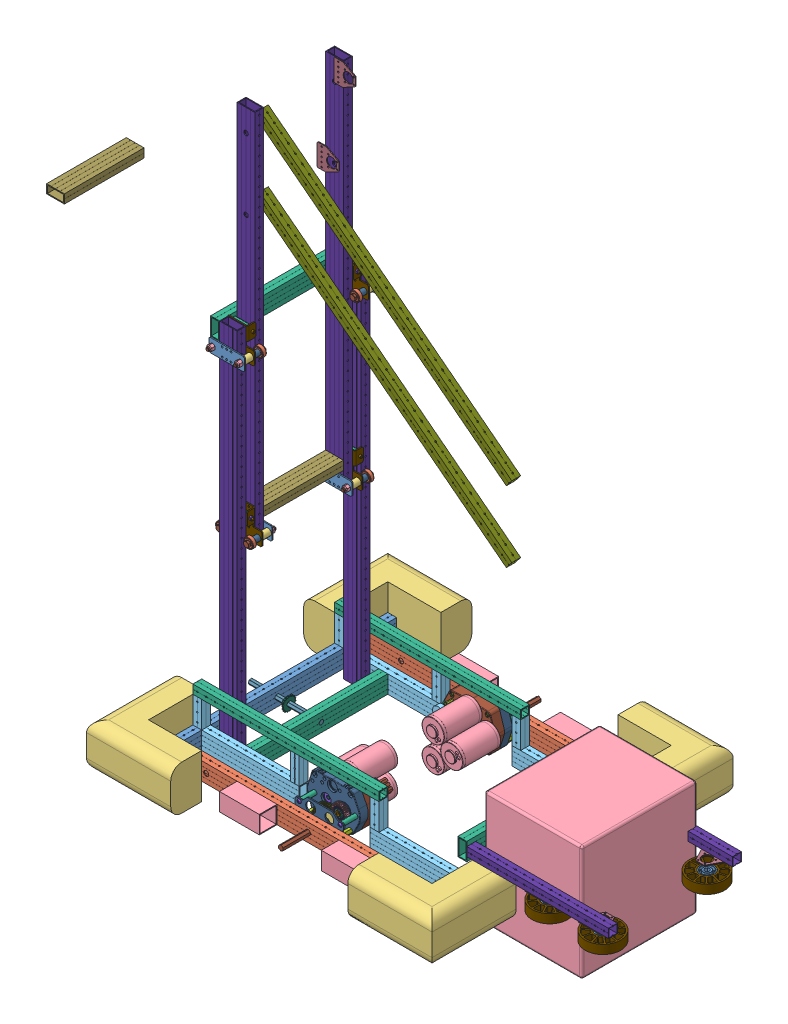
SolidWorks assembly Test Robot 1, configuration Default. Lengths in mm. (continued)
Components (placement in the parent): (continued)
- Elevator Moving Stage-1: Elevator Moving Stage [Default] at (-1117.3569 1209.6863 1583.1183) x (0 0 -1) z (1 0 0) size (614.36 1067.72 354.81)
  - Elevator Fixed Frame-1: Elevator Fixed Frame [Default] at (692.621 1.7594 927.1918) x (1 0 0) z (0 1 0) size (25.4 50.8 1066.8)
  - Elevator Fixed Frame-2: Elevator Fixed Frame [Default] at (438.621 1.7594 927.1918) x (1 0 0) z (0 1 0) size (25.4 50.8 1066.8)
  - Elevator Crossbar-1: Elevator Crossbar [Default] at (1200.621 -252.2406 927.1918) x (0 -1 0) z (-1 0 0) size (25.4 50.8 228.6)
  - am-3844+2x1+Elevator+Assembly+Example-1: am-3844+2x1+Elevator+Assembly+Example [Default] at (298.921 81.9689 954.3698) x (-1 0 0) z (0 0 1) size (82.37 89.82 113.91)
    - Example Single Corner Bearing Assembly-1: Example Single Corner Bearing Assembly [Default] at (-442.3285 289.2703 9.4128) x (0 0 1) z (-1 0 0) size (113.91 89.82 82.37)
      - Large Bearing Block Plate-1: Large Bearing Block Plate [Default] at (-85.6128 70.3392 -35.9285) x (1 0 0) z (0 -1 0) size (101.6 24.99 88.9)
      - Small Bearing Block Plate-1: Small Bearing Block Plate [Default] at (-85.6128 70.3392 -64.5035) x (1 0 0) z (0 -1 0) size (101.6 3.17 38.1)
      - 1614Z Bearing-1: 1614Z Bearing [Default] at (-74.6273 89.3892 -8.941) x (-0.590982 0.806685 0) z (0 0 1) size (28.58 28.58 9.53)
      - 1614Z Bearing-2: 1614Z Bearing [Default] at (5.0017 89.3892 -8.941) x (0.001674 0.999999 0) z (0 0 1) size (28.58 28.58 9.53)
      - AS75-18-64 Aluminum Spacer-1: AS75-18-64 Aluminum Spacer [Default] at (5.0017 89.3892 -35.9285) x (-0.668699 0.743533 0) z (-0.743533 -0.668699 0) size (19.05 25.41 19.05)
      - AS75-18-64 Aluminum Spacer-2: AS75-18-64 Aluminum Spacer [Default] at (-74.6273 89.3892 -61.3285) x (0.536222 0.844077 0) z (0.844077 -0.536222 0) size (19.05 25.41 19.05)
      - 3-8-16 NyLock Nut - Mcm 95615A140_95615A140-1: 3-8-16 NyLock Nut - Mcm 95615A140_95615A140 [Default] at (5.0017 89.3892 -64.5035) x (1 0 0) z (0 1 0) size (14.29 12 16.5)
      - 3-8-16 NyLock Nut - Mcm 95615A140_95615A140-2: 3-8-16 NyLock Nut - Mcm 95615A140_95615A140 [Default] at (-74.6273 89.3892 -64.5035) x (1 0 0) z (0 1 0) size (14.29 12 16.5)
      - am-0602 .250 x .192 x 2.14 Brass Tube-1: am-0602 .250 x .192 x 2.14 Brass Tube [Default] at (-7.6348 38.5892 -20.4599) x (0 0 1) z (-1 0 0) size (6.35 6.35 54.36)
      - 13RS075051 .750 x .260 x 1.00 Spacer-1: 13RS075051 .750 x .260 x 1.00 Spacer [Default] at (-60.2128 38.5892 -20.4599) x (0 -0.722855 0.691) z (0 0.691 0.722855) size (19.05 25.4 19.05)
      - 13RS075051 .750 x .260 x 1.00 Spacer-2: 13RS075051 .750 x .260 x 1.00 Spacer [Default] at (-34.8128 38.5892 -20.4599) x (0 -0.801304 -0.598258) z (0 -0.598258 0.801304) size (19.05 25.4 19.05)
      - 0.25 Flat Washer_Preferred Wide FW 0.25-1: 0.25 Flat Washer_Preferred Wide FW 0.25 [Default] at (-60.2128 38.5892 -20.4599) x (1 0 0) z (0 -0.116572 0.993182) size (1.4 15.88 15.88)
      - 0.25 Flat Washer_Preferred Wide FW 0.25-2: 0.25 Flat Washer_Preferred Wide FW 0.25 [Default] at (-8.0158 38.5892 -20.4599) size (1.4 15.88 15.88)
      - 10-32 Nylock Nut-1: 10-32 Nylock Nut [Default] at (-65.1658 38.5892 -20.4599) x (0 -0.097883 0.995198) z (-1 0 0) size (9.53 11 5.96)
      - SHCS 10-32 x 2.75_HX-SHCS 0.19-32x2.75x0.875-C-1: SHCS 10-32 x 2.75_HX-SHCS 0.19-32x2.75x0.875-C [Default] at (0.3662 38.5892 -20.4599) x (-1 0 0) z (0 0.982583 -0.185827) size (74.68 7.94 7.94)
      - AS62-18-56 Aluminum Spacer-1: AS62-18-56 Aluminum Spacer [Default] at (5.0017 89.3892 -13.7035) x (0.977193 0.212353 0) z (-0.212353 0.977193 0) size (15.88 19.06 15.88)
      - AS62-18-56 Aluminum Spacer-2: AS62-18-56 Aluminum Spacer [Default] at (-74.6273 89.3892 -13.7035) x (1 0 0) z (0 1 0) size (15.88 19.06 15.88)
      - 375-16 x 3 Hex Bolt_HFBOLT 0.375-16x2.5x1-C-1: 375-16 x 3 Hex Bolt_HFBOLT 0.375-16x2.5x1-C [Default] at (-74.6273 89.3892 1.9937) x (0 0 -1) z (1 0 0) size (82.37 16.48 14.28)
      - 375-16 x 3 Hex Bolt_HFBOLT 0.375-16x2.5x1-C-2: 375-16 x 3 Hex Bolt_HFBOLT 0.375-16x2.5x1-C [Default] at (5.0017 89.3892 1.9937) x (0 0 -1) z (-0.5 -0.866025 0) size (82.37 16.48 14.28)
  - am-3844+2x1+Elevator+Assembly+Example-2: am-3844+2x1+Elevator+Assembly+Example [Default] at (832.321 81.9689 900.0138) x (1 0 0) z (0 0 -1) size (82.37 89.82 113.91)
    - Example Single Corner Bearing Assembly-1: Example Single Corner Bearing Assembly [Default] at (-442.3285 289.2703 9.4128) x (0 0 1) z (-1 0 0) size (113.91 89.82 82.37)
      - Large Bearing Block Plate-1: Large Bearing Block Plate [Default] at (-85.6128 70.3392 -35.9285) x (1 0 0) z (0 -1 0) size (101.6 24.99 88.9)
      - Small Bearing Block Plate-1: Small Bearing Block Plate [Default] at (-85.6128 70.3392 -64.5035) x (1 0 0) z (0 -1 0) size (101.6 3.17 38.1)
      - 1614Z Bearing-1: 1614Z Bearing [Default] at (-74.6273 89.3892 -8.941) x (-0.590982 0.806685 0) z (0 0 1) size (28.58 28.58 9.53)
      - 1614Z Bearing-2: 1614Z Bearing [Default] at (5.0017 89.3892 -8.941) x (0.001674 0.999999 0) z (0 0 1) size (28.58 28.58 9.53)
      - AS75-18-64 Aluminum Spacer-1: AS75-18-64 Aluminum Spacer [Default] at (5.0017 89.3892 -35.9285) x (-0.668699 0.743533 0) z (-0.743533 -0.668699 0) size (19.05 25.41 19.05)
      - AS75-18-64 Aluminum Spacer-2: AS75-18-64 Aluminum Spacer [Default] at (-74.6273 89.3892 -61.3285) x (0.536222 0.844077 0) z (0.844077 -0.536222 0) size (19.05 25.41 19.05)
      - 3-8-16 NyLock Nut - Mcm 95615A140_95615A140-1: 3-8-16 NyLock Nut - Mcm 95615A140_95615A140 [Default] at (5.0017 89.3892 -64.5035) x (1 0 0) z (0 1 0) size (14.29 12 16.5)
      - 3-8-16 NyLock Nut - Mcm 95615A140_95615A140-2: 3-8-16 NyLock Nut - Mcm 95615A140_95615A140 [Default] at (-74.6273 89.3892 -64.5035) x (1 0 0) z (0 1 0) size (14.29 12 16.5)
      - am-0602 .250 x .192 x 2.14 Brass Tube-1: am-0602 .250 x .192 x 2.14 Brass Tube [Default] at (-7.6348 38.5892 -20.4599) x (0 0 1) z (-1 0 0) size (6.35 6.35 54.36)
      - 13RS075051 .750 x .260 x 1.00 Spacer-1: 13RS075051 .750 x .260 x 1.00 Spacer [Default] at (-60.2128 38.5892 -20.4599) x (0 -0.722855 0.691) z (0 0.691 0.722855) size (19.05 25.4 19.05)
      - 13RS075051 .750 x .260 x 1.00 Spacer-2: 13RS075051 .750 x .260 x 1.00 Spacer [Default] at (-34.8128 38.5892 -20.4599) x (0 -0.801304 -0.598258) z (0 -0.598258 0.801304) size (19.05 25.4 19.05)
      - 0.25 Flat Washer_Preferred Wide FW 0.25-1: 0.25 Flat Washer_Preferred Wide FW 0.25 [Default] at (-60.2128 38.5892 -20.4599) x (1 0 0) z (0 -0.116572 0.993182) size (1.4 15.88 15.88)
      - 0.25 Flat Washer_Preferred Wide FW 0.25-2: 0.25 Flat Washer_Preferred Wide FW 0.25 [Default] at (-8.0158 38.5892 -20.4599) size (1.4 15.88 15.88)
      - 10-32 Nylock Nut-1: 10-32 Nylock Nut [Default] at (-65.1658 38.5892 -20.4599) x (0 -0.097883 0.995198) z (-1 0 0) size (9.53 11 5.96)
      - SHCS 10-32 x 2.75_HX-SHCS 0.19-32x2.75x0.875-C-1: SHCS 10-32 x 2.75_HX-SHCS 0.19-32x2.75x0.875-C [Default] at (0.3662 38.5892 -20.4599) x (-1 0 0) z (0 0.982583 -0.185827) size (74.68 7.94 7.94)
      - AS62-18-56 Aluminum Spacer-1: AS62-18-56 Aluminum Spacer [Default] at (5.0017 89.3892 -13.7035) x (0.977193 0.212353 0) z (-0.212353 0.977193 0) size (15.88 19.06 15.88)
      - AS62-18-56 Aluminum Spacer-2: AS62-18-56 Aluminum Spacer [Default] at (-74.6273 89.3892 -13.7035) x (1 0 0) z (0 1 0) size (15.88 19.06 15.88)
      - 375-16 x 3 Hex Bolt_HFBOLT 0.375-16x2.5x1-C-1: 375-16 x 3 Hex Bolt_HFBOLT 0.375-16x2.5x1-C [Default] at (-74.6273 89.3892 1.9937) x (0 0 -1) z (1 0 0) size (82.37 16.48 14.28)
      - 375-16 x 3 Hex Bolt_HFBOLT 0.375-16x2.5x1-C-2: 375-16 x 3 Hex Bolt_HFBOLT 0.375-16x2.5x1-C [Default] at (5.0017 89.3892 1.9937) x (0 0 -1) z (-0.5 -0.866025 0) size (82.37 16.48 14.28)
  - VersaFrame Side Bearing Mount-1: VersaFrame Side Bearing Mount [Default] at (677.635 719.3094 968.4668) x (0 -1 0) z (1 0 0) size (63.5 61.91 2.29)
  - Elevator Crossbar-2: Elevator Crossbar [Default] at (878.1872 560.1378 677.8777) x (0 -1 0) z (-1 0 0) size (25.4 50.8 228.6)
  - VersaFrame Side Bearing Mount-2: VersaFrame Side Bearing Mount [Default] at (611.7557 550.5996 986.6483) x (0 -1 0) z (1 0 0) size (63.5 61.91 2.29)
- Frame Crossbar-1: Frame Crossbar [Default] at (-126.6651 401.7853 458.6973) size (25.4 50.8 381)
- Elevator Bottom Shaft-1: Elevator Bottom Shaft [Default] at (-571.1651 401.415 1016.6308) x (0 -0.821487 -0.570227) z (1 0 0) size (14.48 12.67 203.2)
- 18t Aluminum Hub Sprocket 25 Chain-1: 18t Aluminum Hub Sprocket 25 Chain [Default] at (-209.1834 401.3909 1016.614) x (0 0.426315 0.904575) z (1 0 0) size (39.82 39.37 9.18)
- Elevator Arm Section-1: Elevator Arm Section [Default] at (382.6907 1251.378 1093.6973) x (0.611504 0.791241 0) z (-0.791241 0.611504 0) size (25.4 25.4 914.4)
- Elevator Arm Section-2: Elevator Arm Section [Default] at (382.6907 1454.578 1093.6973) x (0.611504 0.791241 0) z (-0.791241 0.611504 0) size (25.4 25.4 914.4)
- PowerUp Cube-1: PowerUp Cube [Default] at (635.4111 592.3615 852.3973) x (1 0 0) z (0 0 -1) size (330.2 279.4 330.2) (hidden)
- Intake Mechanism-1: Intake Mechanism [Default] at (457.0954 282.5183 859.9029) size (433.8 91.36 438.18) (hidden)
  - Frame Crossbar-1: Frame Crossbar [Default] at (76.7157 246.3432 -401.2056) size (25.4 50.8 381)
  - Intake Arm-1: Intake Arm [Default] at (838.7157 246.3432 335.3944) x (0 0 1) z (-1 0 0) size (25.4 25.4 406.4)
  - am-3480+4IN+500Hex+Bore+Compliant+Wheel-1: am-3480+4IN+500Hex+Bore+Compliant+Wheel [Default] at (454.9031 187.3052 310.6703) x (1 0 0) z (0 1 0) size (101.6 101.6 25.74)
    - 4IN Compliant Wheel FINAL Overmold-1: 4IN Compliant Wheel FINAL Overmold [Default] at (-16.2374 3.8509 18.652) size (101.6 101.6 25.74)
    - 2in Wheel Intergrated 0500 HEX Hub-1: 2in Wheel Intergrated 0500 HEX Hub [Default] at (-16.2374 3.8509 5.952) x (-1 0 0) z (0 0 -1) size (41.91 41.91 25.4)
  - VersaFrame Side Bearing Mount-1: VersaFrame Side Bearing Mount [Default] at (438.6657 231.3572 306.8194) x (-1 0 0) z (0 1 0) size (63.5 61.91 2.29)
  - am-3480+4IN+500Hex+Bore+Compliant+Wheel-2: am-3480+4IN+500Hex+Bore+Compliant+Wheel [Default] at (300.5813 187.3052 298.2434) x (0.716102 0 -0.697996) z (0 1 0) size (101.6 101.6 25.74)
    - 4IN Compliant Wheel FINAL Overmold-1: 4IN Compliant Wheel FINAL Overmold [Default] at (-16.2374 3.8509 18.652) size (101.6 101.6 25.74)
    - 2in Wheel Intergrated 0500 HEX Hub-1: 2in Wheel Intergrated 0500 HEX Hub [Default] at (-16.2374 3.8509 5.952) x (-1 0 0) z (0 0 -1) size (41.91 41.91 25.4)
  - VersaFrame Side Bearing Mount-2: VersaFrame Side Bearing Mount [Default] at (286.2657 231.3572 306.8194) x (-1 0 0) z (0 1 0) size (63.5 61.91 2.29)
  - VersaFrame Side Bearing Mount-3: VersaFrame Side Bearing Mount [Default] at (438.6657 231.3572 8.3694) x (1 0 0) z (0 1 0) size (63.5 61.91 2.29)
  - am-3480+4IN+500Hex+Bore+Compliant+Wheel-3: am-3480+4IN+500Hex+Bore+Compliant+Wheel [Default] at (299.1891 187.3052 18.9274) x (0.899512 0 0.436896) z (0 1 0) size (101.6 101.6 25.74)
    - 4IN Compliant Wheel FINAL Overmold-1: 4IN Compliant Wheel FINAL Overmold [Default] at (-16.2374 3.8509 18.652) size (101.6 101.6 25.74)
    - 2in Wheel Intergrated 0500 HEX Hub-1: 2in Wheel Intergrated 0500 HEX Hub [Default] at (-16.2374 3.8509 5.952) x (-1 0 0) z (0 0 -1) size (41.91 41.91 25.4)
  - VersaFrame Side Bearing Mount-4: VersaFrame Side Bearing Mount [Default] at (286.2657 231.3572 8.3694) x (1 0 0) z (0 1 0) size (63.5 61.91 2.29)
  - am-3480+4IN+500Hex+Bore+Compliant+Wheel-4: am-3480+4IN+500Hex+Bore+Compliant+Wheel [Default] at (421.9996 187.3052 7.5191) x (-0.983506 0 0.180877) z (0 1 0) size (101.6 101.6 25.74)
    - 4IN Compliant Wheel FINAL Overmold-1: 4IN Compliant Wheel FINAL Overmold [Default] at (-16.2374 3.8509 18.652) size (101.6 101.6 25.74)
    - 2in Wheel Intergrated 0500 HEX Hub-1: 2in Wheel Intergrated 0500 HEX Hub [Default] at (-16.2374 3.8509 5.952) x (-1 0 0) z (0 0 -1) size (41.91 41.91 25.4)
  - Intake Arm-2: Intake Arm [Default] at (838.7157 246.3432 -20.2056) x (0 0 1) z (-1 0 0) size (25.4 25.4 406.4)
- Intake Support Arm-1: Intake Support Arm [Default] at (1067.2111 528.8615 1169.8973) x (0 0 -1) z (-1 0 0) size (25.4 50.8 203.2) (hidden)
- Intake Upright-1: Intake Upright [Default] at (343.2349 -195.1147 1220.6973) x (0 0 1) z (0 1 0) size (25.4 50.8 127) (hidden)
- Blue Bumper Side-1: Blue Bumper Side [Default] at (635.3349 376.3853 1258.7973) x (0 0 -1) z (1 0 0) size (482.6 127 88.9) (hidden)
- Fence Model-1: Fence Model [Default] at (787.7349 325.5853 585.6973) size (101.6 482.6 863.6) (hidden)
- Intake Mechanism-2: Intake Mechanism [Default] at (-151.5494 825.4024 1175.0918) x (-1 0 0) z (0 0 -1) size (433.8 91.36 438.18) (hidden)
  - Frame Crossbar-1: Frame Crossbar [Default] at (76.7157 246.3432 -401.2056) size (25.4 50.8 381)
  - Intake Arm-1: Intake Arm [Default] at (838.7157 246.3432 335.3944) x (0 0 1) z (-1 0 0) size (25.4 25.4 406.4)
  - am-3480+4IN+500Hex+Bore+Compliant+Wheel-1: am-3480+4IN+500Hex+Bore+Compliant+Wheel [Default] at (454.9031 187.3052 310.6703) x (1 0 0) z (0 1 0) size (101.6 101.6 25.74)
    - 4IN Compliant Wheel FINAL Overmold-1: 4IN Compliant Wheel FINAL Overmold [Default] at (-16.2374 3.8509 18.652) size (101.6 101.6 25.74)
    - 2in Wheel Intergrated 0500 HEX Hub-1: 2in Wheel Intergrated 0500 HEX Hub [Default] at (-16.2374 3.8509 5.952) x (-1 0 0) z (0 0 -1) size (41.91 41.91 25.4)
  - VersaFrame Side Bearing Mount-1: VersaFrame Side Bearing Mount [Default] at (438.6657 231.3572 306.8194) x (-1 0 0) z (0 1 0) size (63.5 61.91 2.29)
  - am-3480+4IN+500Hex+Bore+Compliant+Wheel-2: am-3480+4IN+500Hex+Bore+Compliant+Wheel [Default] at (300.5813 187.3052 298.2434) x (0.716102 0 -0.697996) z (0 1 0) size (101.6 101.6 25.74)
    - 4IN Compliant Wheel FINAL Overmold-1: 4IN Compliant Wheel FINAL Overmold [Default] at (-16.2374 3.8509 18.652) size (101.6 101.6 25.74)
    - 2in Wheel Intergrated 0500 HEX Hub-1: 2in Wheel Intergrated 0500 HEX Hub [Default] at (-16.2374 3.8509 5.952) x (-1 0 0) z (0 0 -1) size (41.91 41.91 25.4)
  - VersaFrame Side Bearing Mount-2: VersaFrame Side Bearing Mount [Default] at (286.2657 231.3572 306.8194) x (-1 0 0) z (0 1 0) size (63.5 61.91 2.29)
  - VersaFrame Side Bearing Mount-3: VersaFrame Side Bearing Mount [Default] at (438.6657 231.3572 8.3694) x (1 0 0) z (0 1 0) size (63.5 61.91 2.29)
  - am-3480+4IN+500Hex+Bore+Compliant+Wheel-3: am-3480+4IN+500Hex+Bore+Compliant+Wheel [Default] at (299.1891 187.3052 18.9274) x (0.899512 0 0.436896) z (0 1 0) size (101.6 101.6 25.74)
    - 4IN Compliant Wheel FINAL Overmold-1: 4IN Compliant Wheel FINAL Overmold [Default] at (-16.2374 3.8509 18.652) size (101.6 101.6 25.74)
    - 2in Wheel Intergrated 0500 HEX Hub-1: 2in Wheel Intergrated 0500 HEX Hub [Default] at (-16.2374 3.8509 5.952) x (-1 0 0) z (0 0 -1) size (41.91 41.91 25.4)
  - VersaFrame Side Bearing Mount-4: VersaFrame Side Bearing Mount [Default] at (286.2657 231.3572 8.3694) x (1 0 0) z (0 1 0) size (63.5 61.91 2.29)
  - am-3480+4IN+500Hex+Bore+Compliant+Wheel-4: am-3480+4IN+500Hex+Bore+Compliant+Wheel [Default] at (421.9996 187.3052 7.5191) x (-0.983506 0 0.180877) z (0 1 0) size (101.6 101.6 25.74)
    - 4IN Compliant Wheel FINAL Overmold-1: 4IN Compliant Wheel FINAL Overmold [Default] at (-16.2374 3.8509 18.652) size (101.6 101.6 25.74)
    - 2in Wheel Intergrated 0500 HEX Hub-1: 2in Wheel Intergrated 0500 HEX Hub [Default] at (-16.2374 3.8509 5.952) x (-1 0 0) z (0 0 -1) size (41.91 41.91 25.4)
  - Intake Arm-2: Intake Arm [Default] at (838.7157 246.3432 -20.2056) x (0 0 1) z (-1 0 0) size (25.4 25.4 406.4)
- Intake Mechanism-3: Intake Mechanism [Default] at (454.9829 284.4022 910.7029) size (433.8 91.36 438.18)
  - Frame Crossbar-1: Frame Crossbar [Default] at (76.7157 246.3432 -401.2056) size (25.4 50.8 381)
  - Intake Arm-1: Intake Arm [Default] at (838.7157 246.3432 335.3944) x (0 0 1) z (-1 0 0) size (25.4 25.4 406.4)
  - am-3480+4IN+500Hex+Bore+Compliant+Wheel-1: am-3480+4IN+500Hex+Bore+Compliant+Wheel [Default] at (454.9031 187.3052 310.6703) x (1 0 0) z (0 1 0) size (101.6 101.6 25.74)
    - 4IN Compliant Wheel FINAL Overmold-1: 4IN Compliant Wheel FINAL Overmold [Default] at (-16.2374 3.8509 18.652) size (101.6 101.6 25.74)
    - 2in Wheel Intergrated 0500 HEX Hub-1: 2in Wheel Intergrated 0500 HEX Hub [Default] at (-16.2374 3.8509 5.952) x (-1 0 0) z (0 0 -1) size (41.91 41.91 25.4)
  - VersaFrame Side Bearing Mount-1: VersaFrame Side Bearing Mount [Default] at (438.6657 231.3572 306.8194) x (-1 0 0) z (0 1 0) size (63.5 61.91 2.29)
  - am-3480+4IN+500Hex+Bore+Compliant+Wheel-2: am-3480+4IN+500Hex+Bore+Compliant+Wheel [Default] at (300.5813 187.3052 298.2434) x (0.716102 0 -0.697996) z (0 1 0) size (101.6 101.6 25.74)
    - 4IN Compliant Wheel FINAL Overmold-1: 4IN Compliant Wheel FINAL Overmold [Default] at (-16.2374 3.8509 18.652) size (101.6 101.6 25.74)
    - 2in Wheel Intergrated 0500 HEX Hub-1: 2in Wheel Intergrated 0500 HEX Hub [Default] at (-16.2374 3.8509 5.952) x (-1 0 0) z (0 0 -1) size (41.91 41.91 25.4)
  - VersaFrame Side Bearing Mount-2: VersaFrame Side Bearing Mount [Default] at (286.2657 231.3572 306.8194) x (-1 0 0) z (0 1 0) size (63.5 61.91 2.29)
  - VersaFrame Side Bearing Mount-3: VersaFrame Side Bearing Mount [Default] at (438.6657 231.3572 8.3694) x (1 0 0) z (0 1 0) size (63.5 61.91 2.29)
  - am-3480+4IN+500Hex+Bore+Compliant+Wheel-3: am-3480+4IN+500Hex+Bore+Compliant+Wheel [Default] at (299.1891 187.3052 18.9274) x (0.899512 0 0.436896) z (0 1 0) size (101.6 101.6 25.74)
    - 4IN Compliant Wheel FINAL Overmold-1: 4IN Compliant Wheel FINAL Overmold [Default] at (-16.2374 3.8509 18.652) size (101.6 101.6 25.74)
    - 2in Wheel Intergrated 0500 HEX Hub-1: 2in Wheel Intergrated 0500 HEX Hub [Default] at (-16.2374 3.8509 5.952) x (-1 0 0) z (0 0 -1) size (41.91 41.91 25.4)
  - VersaFrame Side Bearing Mount-4: VersaFrame Side Bearing Mount [Default] at (286.2657 231.3572 8.3694) x (1 0 0) z (0 1 0) size (63.5 61.91 2.29)
  - am-3480+4IN+500Hex+Bore+Compliant+Wheel-4: am-3480+4IN+500Hex+Bore+Compliant+Wheel [Default] at (421.9996 187.3052 7.5191) x (-0.983506 0 0.180877) z (0 1 0) size (101.6 101.6 25.74)
    - 4IN Compliant Wheel FINAL Overmold-1: 4IN Compliant Wheel FINAL Overmold [Default] at (-16.2374 3.8509 18.652) size (101.6 101.6 25.74)
    - 2in Wheel Intergrated 0500 HEX Hub-1: 2in Wheel Intergrated 0500 HEX Hub [Default] at (-16.2374 3.8509 5.952) x (-1 0 0) z (0 0 -1) size (41.91 41.91 25.4)
  - Intake Arm-2: Intake Arm [Default] at (838.7157 246.3432 -20.2056) x (0 0 1) z (-1 0 0) size (25.4 25.4 406.4)
- Intake Upright 2-1: Intake Upright 2 [Default] at (518.9986 1178.4455 865.0973) x (0 0 -1) z (0 -1 0) size (25.4 50.8 127)
- VersaFrame Corner Gusset-1: VersaFrame Corner Gusset [Default] at (546.4349 427.1853 826.9973) x (-1 0 0) z (0 0 -1) size (69.72 69.72 25.4)
- PowerUp Cube-2: PowerUp Cube [Default] at (544.3986 326.2755 877.7973) x (0 1 0) z (0 0 -1) size (330.2 279.4 330.2)
- Assem2^Test Robot 1-1: Assem2^Test Robot 1 [Default] at origin size (533.4 101.6 25.4) (virtual)
  - Superstructure Upright-1: Superstructure Upright [Default] at (-253.6651 -245.9147 814.2973) x (0 0 -1) z (0 1 0) size (25.4 25.4 76.2)
  - Superstructure Crossbar-1: Superstructure Crossbar [Default] at (-482.2651 516.0853 814.2973) x (0 0 -1) z (1 0 0) size (25.4 25.4 533.4)
  - Superstructure Upright-2: Superstructure Upright [Default] at (254.3349 -245.9147 814.2973) x (0 0 -1) z (0 1 0) size (25.4 25.4 76.2)
  - Superstructure Upright-3: Superstructure Upright [Default] at (25.7349 -245.9147 814.2973) x (0 0 -1) z (0 1 0) size (25.4 25.4 76.2)
- Assem2^Test Robot 1-2: Assem2^Test Robot 1 [Default] at (0 0 406.4) size (533.4 101.6 25.4) (virtual)
  - Superstructure Upright-1: Superstructure Upright [Default] at (-253.6651 -245.9147 814.2973) x (0 0 -1) z (0 1 0) size (25.4 25.4 76.2)
  - Superstructure Crossbar-1: Superstructure Crossbar [Default] at (-482.2651 516.0853 814.2973) x (0 0 -1) z (1 0 0) size (25.4 25.4 533.4)
  - Superstructure Upright-2: Superstructure Upright [Default] at (254.3349 -245.9147 814.2973) x (0 0 -1) z (0 1 0) size (25.4 25.4 76.2)
  - Superstructure Upright-3: Superstructure Upright [Default] at (25.7349 -245.9147 814.2973) x (0 0 -1) z (0 1 0) size (25.4 25.4 76.2)
Mates (geometry in assembly coordinates):
- Coincident3: coincident anti-aligned: plane of Test Base 1-1/Base Side Rail Internal-4 through (-240.9651 376.3853 1207.9973) normal (0 0 -1); plane of Elevator Base Frame-1/Elevator Fixed Frame-1 through (-215.5651 1443.1853 1207.9973) normal (0 0 1)
- Distance2: distance = 25.4 mm anti-aligned: plane of Test Base 1-1/Base Rear Rail-1 through (-240.9651 376.3853 1360.3973) normal (1 0 0); plane of Elevator Base Frame-1/Elevator Fixed Frame-1 through (-215.5651 1443.1853 1182.5973) normal (-1 0 0)
- Coincident5: coincident aligned: plane of Test Base 1-1/Base Rear Rail-1 through (-266.3651 376.3853 1360.3973) normal (0 -1 0); plane of Elevator Base Frame-1/Elevator Fixed Frame-1 through (-190.1651 376.3853 1195.2973) normal (0 -1 0)
- Distance6: distance = 25.4 mm anti-aligned: plane of Elevator Moving Stage-1/Elevator Fixed Frame-1 through (-164.7651 1960.7457 877.7973) normal (0 0 -1); plane of Elevator Base Frame-1/Elevator Fixed Frame-2 through (-215.5651 1443.1853 852.3973) normal (0 0 1)
- Coincident11: coincident aligned: plane of Elevator Base Frame-1/Elevator Fixed Frame-1 through (-164.7651 1443.1853 1182.5973) normal (1 0 0); plane of Elevator Moving Stage-1/Elevator Fixed Frame-2 through (-164.7651 1960.7457 1157.1973) normal (1 0 0)
- LimitDistance1: limit distance = 517.5603 mm aligned: plane of Elevator Base Frame-1/Elevator Fixed Frame-1 through (-190.1651 1443.1853 1195.2973) normal (0 1 0); plane of Elevator Moving Stage-1/Elevator Fixed Frame-2 through (-190.1651 1960.7457 1144.4973) normal (0 1 0)
- Coincident14: coincident aligned: plane of Test Base 1-1/Base Side Rail Internal-4 through (-240.9651 427.1853 1207.9973) normal (0 1 0); plane of Frame Crossbar-1 through (-139.3651 427.1853 -290.6027) normal (0 1 0)
- Coincident15: coincident anti-aligned: plane of Test Base 1-1/Base Side Rail Internal-4 through (-240.9651 376.3853 1207.9973) normal (0 0 -1); plane of Frame Crossbar-1 through (-139.3651 427.1853 1207.9973) normal (0 0 1)
- Distance8: distance = 25.4 mm anti-aligned: plane of Elevator Base Frame-1/Elevator Fixed Frame-1 through (-164.7651 1443.1853 1182.5973) normal (1 0 0); plane of Frame Crossbar-1 through (-139.3651 401.7853 458.6973) normal (-1 0 0)
- Coincident17: coincident aligned: plane of Frame Crossbar-1 through (-113.9651 401.7853 458.6973) normal (1 0 0); plane of Elevator Bottom Shaft-1 through (-113.9651 395.4036 1012.458) normal (1 0 0)
- Tangent7: tangent: cylinder of Frame Crossbar-1 through (-63.1651 401.8615 1017.4973) axis (-1 0 0) radius 6.35; line of Elevator Bottom Shaft-1 through (-113.9651 407.4507 1020.5112) axis (-1 0 0)
- Tangent8: tangent: cylinder of Frame Crossbar-1 through (-63.1651 401.8615 1017.4973) axis (-1 0 0) radius 6.35; line of Elevator Bottom Shaft-1 through (-113.9651 401.0723 1023.7981) axis (-1 0 0)
- Coincident18: coincident anti-aligned: plane of Elevator Bottom Shaft-1 through (-113.9651 408.0344 1013.5111) normal (0 0.996542 0.083088); plane of 18t Aluminum Hub Sprocket 25 Chain-1 through (-215.5661 408.0368 1013.4819) normal (0 -0.996542 -0.083088)
- Coincident19: coincident anti-aligned: plane of Elevator Bottom Shaft-1 through (-113.9651 407.4264 1020.8035) normal (0 0.426315 0.904575); plane of 18t Aluminum Hub Sprocket 25 Chain-1 through (-215.5661 407.4264 1020.8035) normal (0 -0.426315 -0.904575)
- Distance9: distance = 25.4 mm anti-aligned: plane of Test Base 1-1/Base Rear Rail-1 through (-240.9651 376.3853 1360.3973) normal (1 0 0); plane of 18t Aluminum Hub Sprocket 25 Chain-1 through (-215.5651 401.3909 1016.614) normal (-1 0 0)
- Concentric1: concentric anti-aligned: cylinder of Elevator Moving Stage-1/Elevator Fixed Frame-2 through (-190.0889 1694.0457 877.7972) axis (0 0 1) radius 6.35; cylinder of Elevator Arm Section-1 through (-190.0889 1694.0457 1106.3973) axis (0 0 -1) radius 2.0701
- Distance11: distance = 25.4 mm anti-aligned: plane of Elevator Moving Stage-1/Elevator Fixed Frame-2 through (-164.7651 1960.7457 1131.7973) normal (0 0 -1); plane of Elevator Arm Section-1 through (-217.9525 1699.5291 1106.3973) normal (0 0 1)
- Coincident20: coincident aligned: plane of Elevator Arm Section-1 through (-217.9525 1699.5291 1106.3973) normal (0 0 1); plane of Elevator Arm Section-2 through (-217.9525 1902.7291 1106.3973) normal (0 0 1)
- Angle3: planar angle = 0 rad aligned: plane of Elevator Arm Section-1 through (-202.4203 1719.6266 1106.3973) normal (0.611504 0.791241 0); plane of Elevator Arm Section-2 through (-202.4203 1922.8266 1106.3973) normal (0.611504 0.791241 0)
- Concentric2: concentric anti-aligned: cylinder of Elevator Moving Stage-1/Elevator Fixed Frame-2 through (-190.0889 1897.2457 877.7972) axis (0 0 1) radius 6.35; cylinder of Elevator Arm Section-2 through (-190.0889 1897.2457 1106.3973) axis (0 0 -1) radius 2.0701
- LimitAngle3: limit planar angle = 1.047198 rad aligned: plane of Elevator Arm Section-2; plane of ? through (-190.1651 1443.1853 1131.7973) normal (0 1 0)
- Coincident23: coincident aligned: plane of Test Base 1-1/Base Side Rail Internal-2 through (521.0349 376.3853 1233.3973) normal (0 0 1); plane of Intake Upright-1 through (343.2349 -195.1147 1233.3973) normal (0 0 1)
- Coincident24: coincident anti-aligned: plane of Test Base 1-1/Base Side Rail Internal-2 through (521.0349 427.1853 1233.3973) normal (0 1 0); plane of Intake Upright-1 through (343.2349 427.1853 1220.6973) normal (0 -1 0)
- Concentric3: concentric anti-aligned: cylinder of Intake Support Arm-1 through (343.3111 528.7853 1182.5973) axis (0 0 -1) radius 6.35; cylinder of Intake Upright-1 through (343.3111 528.7853 1207.9973) axis (0 0 1) radius 6.35
- Distance13: distance = 25.4 mm anti-aligned: plane of Intake Upright-1 through (343.2349 -195.1147 1207.9973) normal (0 0 -1); plane of Intake Support Arm-1 through (1067.2111 528.8615 1182.5973) normal (0 0 1)
- LimitAngle5: limit planar angle = 0 rad aligned: plane of Intake Support Arm-1 through (317.9111 554.2615 1182.5973) normal (0 1 0); plane of Intake Upright-1 through (368.6349 554.1853 1207.9973) normal (0 1 0)
- Distance14: distance = 76.2 mm aligned: plane of Intake Upright-1 through (317.8349 554.1853 1207.9973) normal (-1 0 0); plane of Test Base 1-1/Base Side Rail Internal-2 through (241.6349 401.7853 1220.6973) normal (-1 0 0)
- Coincident25: coincident aligned: plane of Intake Mechanism-1/Frame Crossbar-1 through (521.1111 554.2615 -290.6027) normal (0 1 0); plane of Intake Support Arm-1 through (317.9111 554.2615 1182.5973) normal (0 1 0)
- Coincident26: coincident anti-aligned: plane of Intake Mechanism-1/Frame Crossbar-1 through (521.1111 528.8615 458.6973) normal (-1 0 0); plane of Intake Support Arm-1 through (521.1111 528.8615 1169.8973) normal (1 0 0)
- Distance16: distance = 25.4 mm aligned: plane of Intake Support Arm-1 through (1067.2111 528.8615 1182.5973) normal (0 0 1); plane of Intake Mechanism-1/Frame Crossbar-1 through (521.1111 554.2615 1207.9973) normal (0 0 1)
- Distance20: distance = 50.8 mm aligned: plane of PowerUp Cube-1 through (635.4111 592.3615 852.3973) normal (0 1 0); plane of Intake Mechanism-1/Intake Arm-1 through (546.5111 541.5615 1182.5973) normal (0 1 0)
- Distance21: distance = 88.9 mm anti-aligned: plane of Intake Mechanism-1/Frame Crossbar-1 through (546.5111 528.8615 458.6973) normal (1 0 0); plane of PowerUp Cube-1 through (635.4111 312.9615 852.3973) normal (-1 0 0)
- Coincident27: coincident anti-aligned: plane of PowerUp Cube-1 through (635.4111 312.9615 1182.5973) normal (0 0 1); plane of Intake Mechanism-1/Intake Arm-1 through (546.5111 516.1615 1182.5973) normal (0 0 -1)
- Distance23: distance = 152.4 mm anti-aligned: plane of Test Base 1-1/Blue Bumper-1 through (635.3349 503.3853 1449.2973) normal (1 0 0); plane of Fence Model-1 through (787.7349 325.5853 1449.2973) normal (-1 0 0)
- Coincident29: coincident aligned: plane of Test Base 1-1/Blue Bumper-1 through (635.3349 503.3853 1449.2973) normal (0 0 1); plane of Fence Model-1 through (787.7349 325.5853 1449.2973) normal (0 0 1)
- Distance22: distance = 50.8 mm aligned: plane of Fence Model-1 through (787.7349 325.5853 1449.2973) normal (0 -1 0); plane of Test Base 1-1/Blue Bumper-1 through (635.3349 376.3853 1449.2973) normal (0 -1 0)
- Coincident30: coincident anti-aligned: plane of Elevator Moving Stage-1/Elevator Fixed Frame-2 through (-215.5651 1960.7457 1157.1973) normal (-1 0 0); plane of Intake Mechanism-2/Frame Crossbar-1 through (-215.5651 1071.7457 1576.2973) normal (1 0 0)
- Coincident31: coincident aligned: plane of Elevator Base Frame-1/Elevator Fixed Frame-1 through (-215.5651 1443.1853 1207.9973) normal (0 0 1); plane of Intake Mechanism-2/Intake Arm-2 through (-240.9651 1059.0457 1207.9973) normal (0 0 1)
- Distance25: distance = 76.2 mm: line of Elevator Moving Stage-1/Elevator Crossbar-1 through (-202.9413 970.1457 903.1973) axis (0 0 1); plane of Intake Mechanism-2/Frame Crossbar-1 through (-215.5651 1046.3457 826.9973) normal (0 -1 0)
- Coincident35: coincident anti-aligned: plane of Test Base 1-1/Frame Crossbar-1 through (546.4349 401.7853 458.6973) normal (1 0 0); plane of Blue Bumper Side-1 through (546.4349 376.3853 776.1973) normal (-1 0 0)
- Coincident36: coincident aligned: plane of Test Base 1-1/Frame Crossbar-1 through (521.0349 376.3853 1207.9973) normal (0 -1 0); plane of Blue Bumper Side-1 through (635.3349 376.3853 776.1973) normal (0 -1 0)
- Distance26: distance = 50.8 mm anti-aligned: plane of Blue Bumper Side-1 through (635.3349 376.3853 1258.7973) normal (0 0 1); plane of Test Base 1-1/Base Side Rail Internal-2 through (521.0349 376.3853 1207.9973) normal (0 0 -1)
- Coincident37: coincident aligned: plane of Test Base 1-1/Frame Crossbar-1 through (546.4349 401.7853 458.6973) normal (1 0 0); plane of VersaFrame Corner Gusset-1 through (546.4349 427.1853 826.9973) normal (1 0 0)
- Coincident38: coincident aligned: plane of Test Base 1-1/Base Side Rail Internal-1 through (521.0349 376.3853 826.9973) normal (0 0 1); plane of VersaFrame Corner Gusset-1 through (546.4349 427.1853 826.9973) normal (0 0 1)
- Coincident39: coincident anti-aligned: plane of Test Base 1-1/Base Side Rail Internal-1 through (521.0349 427.1853 826.9973) normal (0 1 0); plane of VersaFrame Corner Gusset-1 through (546.4349 427.1853 826.9973) normal (0 -1 0)
- Concentric4: concentric anti-aligned: cylinder of Intake Upright 2-1 through (519.0748 454.5455 877.7973) axis (0 0 -1) radius 6.35; cylinder of VersaFrame Corner Gusset-1 through (519.0748 454.5455 823.8223) axis (0 0 1) radius 14.2875
- Distance27: distance = 25.4 mm anti-aligned: plane of VersaFrame Corner Gusset-1 through (546.4349 427.1853 826.9973) normal (0 0 1); plane of Intake Upright 2-1 through (518.9986 1178.4455 852.3973) normal (0 0 -1)
- Distance29: distance = 25.4 mm anti-aligned: plane of PowerUp Cube-2 through (823.7986 326.2755 1207.9973) normal (0 0 1); plane of Intake Mechanism-3/Intake Arm-1 through (544.3986 518.0455 1233.3973) normal (0 0 -1)
- Coincident42: coincident anti-aligned: plane of Intake Mechanism-3/Frame Crossbar-1 through (544.3986 530.7455 509.4973) normal (1 0 0); plane of PowerUp Cube-2 through (544.3986 326.2755 877.7973) normal (-1 0 0)
- Distance30: distance = 191.77 mm aligned: plane of PowerUp Cube-2 through (823.7986 326.2755 877.7973) normal (0 -1 0); plane of Intake Mechanism-3/Intake Arm-1 through (544.3986 518.0455 1233.3973) normal (0 -1 0)
- LimitAngle8: limit planar angle = 0 rad aligned: plane of Test Base 1-1/Base Side Rail Internal-1 through (521.0349 427.1853 826.9973) normal (0 1 0); plane of Intake Upright 2-1 through (518.9986 556.1455 865.0973) normal (0 1 0)
- Coincident43: coincident aligned: plane of Intake Mechanism-3/Frame Crossbar-1 through (518.9986 556.1455 -239.8027) normal (0 1 0); plane of Intake Upright 2-1 through (518.9986 556.1455 865.0973) normal (0 1 0)
- Coincident45: coincident anti-aligned: plane of Intake Mechanism-3/Frame Crossbar-1 through (531.6986 530.7455 877.7973) normal (0 0 -1); plane of Intake Upright 2-1 through (518.9986 1178.4455 877.7973) normal (0 0 1)
- Coincident46: coincident aligned: plane of Intake Mechanism-3/Frame Crossbar-1 through (544.3986 530.7455 509.4973) normal (1 0 0); plane of Intake Upright 2-1 through (544.3986 1927.7455 877.7973) normal (1 0 0)
- Coincident64: coincident anti-aligned: plane of Test Base 1-1/Base Rear Rail-1 through (-266.3651 427.1853 1360.3973) normal (0 1 0); plane of Assem2^Test Robot 1-1/Superstructure Upright-1 through (-253.6651 427.1853 814.2973) normal (0 -1 0)
- Coincident65: coincident aligned: plane of Test Base 1-1/Base Side Rail Internal-3 through (-240.9651 376.3853 801.5973) normal (0 0 -1); plane of Assem2^Test Robot 1-1/Superstructure Upright-1 through (-240.9651 503.3853 801.5973) normal (0 0 -1)
- Coincident66: coincident aligned: plane of Test Base 1-1/Base Rear Rail-1 through (-266.3651 376.3853 1360.3973) normal (-1 0 0); plane of Assem2^Test Robot 1-1/Superstructure Upright-1 through (-266.3651 503.3853 826.9973) normal (-1 0 0)
- Coincident67: coincident aligned: plane of Test Base 1-1/Base Rear Rail-1 through (-266.3651 376.3853 1360.3973) normal (-1 0 0); plane of Assem2^Test Robot 1-2/Superstructure Upright-1 through (-266.3651 503.3853 1233.3973) normal (-1 0 0)
- Coincident68: coincident aligned: plane of Test Base 1-1/Base Side Rail Internal-4 through (-240.9651 376.3853 1207.9973) normal (0 0 -1); plane of Assem2^Test Robot 1-2/Superstructure Upright-1 through (-240.9651 503.3853 1207.9973) normal (0 0 -1)
- Coincident69: coincident anti-aligned: plane of Test Base 1-1/Base Rear Rail-1 through (-266.3651 427.1853 1360.3973) normal (0 1 0); plane of Assem2^Test Robot 1-2/Superstructure Upright-1 through (-253.6651 427.1853 1220.6973) normal (0 -1 0)
